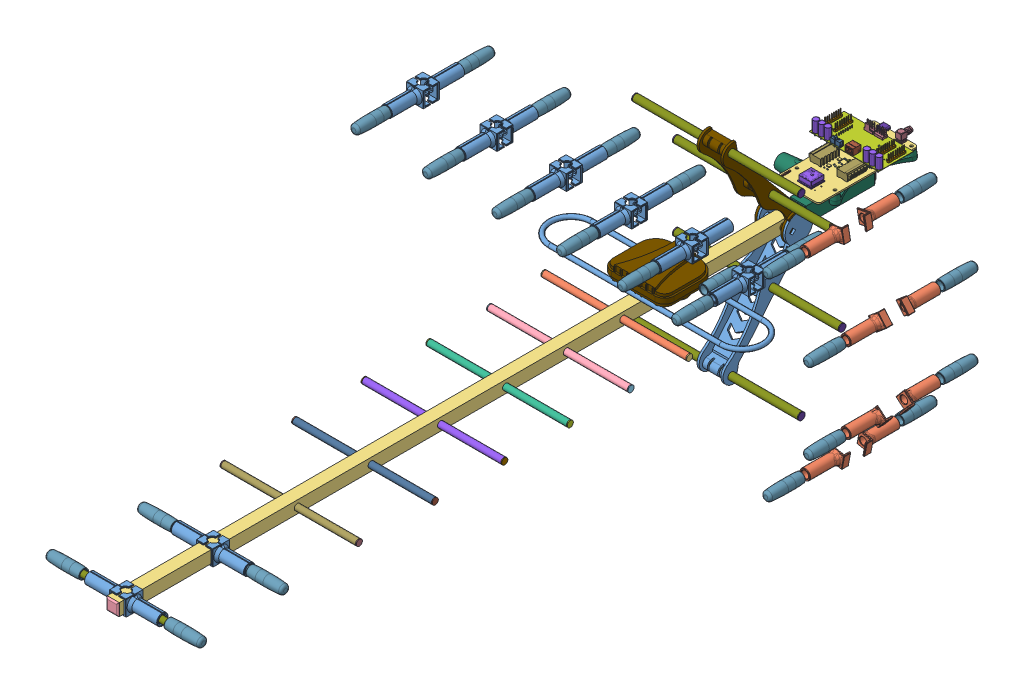
SolidWorks assembly 1. 868MHz Yagi Assembly, configuration Default. Lengths in mm.
Overall size (806.01 707.25 920.96).
274 component instances, 76 part files, 216 mates.
Components (placement in the parent):
- antenna sheath-1: antenna sheath [Default] at (505.0614 466.1407 652.9384) x (0 1 0) z (0 0 1) size (18 10 41)
- antenna sheath-2: antenna sheath [Default] at (505.0614 466.1407 652.9384) x (0 -1 0) z (0 0 1) size (18 10 41)
- antenna sheath-3: antenna sheath [Default] at (440.0614 466.1407 652.9384) x (0 1 0) z (0 0 1) size (18 10 41)
- antenna sheath-4: antenna sheath [Default] at (440.0614 466.1407 652.9384) x (0 -1 0) z (0 0 1) size (18 10 41)
- antenna sheath-5: antenna sheath [Default] at (370.0614 466.1407 652.9384) x (0 -1 0) z (0 0 1) size (18 10 41)
- antenna sheath-6: antenna sheath [Default] at (370.0614 466.1407 652.9384) x (0 1 0) z (0 0 1) size (18 10 41)
- antenna sheath-7: antenna sheath [Default] at (295.0614 466.1407 652.9384) x (0 1 0) z (0 0 1) size (18 10 41)
- antenna sheath-8: antenna sheath [Default] at (295.0614 466.1407 652.9384) x (0 -1 0) z (0 0 1) size (18 10 41)
- antenna sheath-9: antenna sheath [Default] at (215.0614 466.1407 652.9384) x (0 1 0) z (0 0 1) size (18 10 41)
- antenna sheath-10: antenna sheath [Default] at (215.0614 466.1407 652.9384) x (0 -1 0) z (0 0 1) size (18 10 41)
- antenna sheath-11: antenna sheath [Default] at (130.0614 466.1407 652.9384) x (0 1 0) z (0 0 1) size (18 10 41)
- antenna sheath-12: antenna sheath [Default] at (130.0614 466.1407 652.9384) x (0 -1 0) z (0 0 1) size (18 10 41)
- antenna sheath-13: antenna sheath [Default] at (7 0 757.5) x (0 1 0) z (1 0 0) size (18 10 41)
- antenna sheath-14: antenna sheath [Default] at (7 0 757.5) x (0 -1 0) z (1 0 0) size (18 10 41)
- antenna sheath-15: antenna sheath [Default] at (7 0 857.5) x (0 -1 0) z (1 0 0) size (18 10 41)
- antenna sheath-16: antenna sheath [Default] at (7 0 857.5) x (0 1 0) z (1 0 0) size (18 10 41)
- antenna sheath-17: antenna sheath [Default] at (505.0614 466.1407 638.9384) x (0 -1 0) z (0 0 -1) size (18 10 41)
- antenna sheath-18: antenna sheath [Default] at (505.0614 466.1407 638.9384) x (0 1 0) z (0 0 -1) size (18 10 41)
- antenna sheath-19: antenna sheath [Default] at (440.0614 466.1407 638.9384) x (0 -1 0) z (0 0 -1) size (18 10 41)
- antenna sheath-20: antenna sheath [Default] at (440.0614 466.1407 638.9384) x (0 1 0) z (0 0 -1) size (18 10 41)
- antenna sheath-21: antenna sheath [Default] at (370.0614 466.1407 638.9384) x (0 -1 0) z (0 0 -1) size (18 10 41)
- antenna sheath-22: antenna sheath [Default] at (370.0614 466.1407 638.9384) x (0 1 0) z (0 0 -1) size (18 10 41)
- antenna sheath-23: antenna sheath [Default] at (295.0614 466.1407 638.9384) x (0 1 0) z (0 0 -1) size (18 10 41)
- antenna sheath-24: antenna sheath [Default] at (295.0614 466.1407 638.9384) x (0 -1 0) z (0 0 -1) size (18 10 41)
- antenna sheath-25: antenna sheath [Default] at (215.0614 466.1407 638.9384) x (0 -1 0) z (0 0 -1) size (18 10 41)
- antenna sheath-26: antenna sheath [Default] at (215.0614 466.1407 638.9384) x (0 1 0) z (0 0 -1) size (18 10 41)
- antenna sheath-27: antenna sheath [Default] at (130.0614 466.1407 638.9384) x (0 1 0) z (0 0 -1) size (18 10 41)
- antenna sheath-28: antenna sheath [Default] at (130.0614 466.1407 638.9384) x (0 -1 0) z (0 0 -1) size (18 10 41)
- antenna sheath-29: antenna sheath [Default] at (-7 0 757.5) x (0 -1 0) z (-1 0 0) size (18 10 41)
- antenna sheath-30: antenna sheath [Default] at (-7 0 757.5) x (0 1 0) z (-1 0 0) size (18 10 41)
- antenna sheath-31: antenna sheath [Default] at (-7 0 857.5) x (0 1 0) z (-1 0 0) size (18 10 41)
- antenna sheath-32: antenna sheath [Default] at (-7 0 857.5) x (0 -1 0) z (-1 0 0) size (18 10 41)
- ground plane sheath-1: ground plane sheath [Default] at (622.1186 354.933 628.9384) x (0.186459 0.982463 0) z (0 0 -1) size (15.31 15.12 43)
- ground plane sheath-2: ground plane sheath [Default] at (622.1186 354.933 662.9384) x (-0.186459 -0.982463 0) z (0 0 1) size (15.31 15.12 43)
- ground plane sheath-3: ground plane sheath [Default] at (669.0995 419.8148 662.9384) x (-0.642788 -0.766044 0) z (0 0 1) size (15.31 15.12 43)
- ground plane sheath-4: ground plane sheath [Default] at (669.0995 419.8148 628.9384) x (0.642788 0.766044 0) z (0 0 -1) size (15.31 15.12 43)
- ground plane sheath-5: ground plane sheath [Default] at (669.0995 512.4667 662.9384) x (0.642788 -0.766044 0) z (0 0 1) size (15.31 15.12 43)
- ground plane sheath-6: ground plane sheath [Default] at (669.0995 512.4667 628.9384) x (-0.642788 0.766044 0) z (0 0 -1) size (15.31 15.12 43)
- ground plane sheath-7: ground plane sheath [Default] at (622.1186 577.3485 662.9384) x (0.186459 -0.982463 0) z (0 0 1) size (15.31 15.12 43)
- ground plane sheath-8: ground plane sheath [Default] at (622.1186 577.3485 628.9384) x (-0.186459 0.982463 0) z (0 0 -1) size (15.31 15.12 43)
- Main_Board_1_1-1: Main_Board_1_1 [Default] at (36 19.75 -38.9645) x (-1 0 0) z (0 1 0) size (70 133 15.95)
  - Main_Board_1_1_BOARD-1: Main_Board_1_1_BOARD [Default] at origin size (52 115 1.63)
  - BMP581_CMP-048-000000-2-1: BMP581_CMP-048-000000-2 [Default] at (43 50.5 0.0203) x (-0.707107 -0.707107 0) z (0 0 -1) size (2 2 0.8)
  - BMP581_CMP-048-000000-2-2: BMP581_CMP-048-000000-2 [Default] at (45.5 45.5 1.6065) x (0.707107 -0.707107 0) z (0 0 1) size (2 2 0.8)
  - RESC1609X50X30ML8T20_CMP-009-00185-4-1: RESC1609X50X30ML8T20_CMP-009-00185-4 [Default] at (40.25 53.25 0.0203) x (0 1 0) z (0 0 -1) size (1.65 0.95 0.5)
  - RESC1609X50X30ML8T20_CMP-009-00185-4-2: RESC1609X50X30ML8T20_CMP-009-00185-4 [Default] at (47.5 49 0.0203) x (0 1 0) z (0 0 -1) size (1.65 0.95 0.5)
  - RESC1609X50X30ML8T20_CMP-009-00185-4-3: RESC1609X50X30ML8T20_CMP-009-00185-4 [Default] at (41.5 53.25 0.0203) x (0 1 0) z (0 0 -1) size (1.65 0.95 0.5)
  - RESC1609X50X30ML8T20_CMP-009-00185-4-4: RESC1609X50X30ML8T20_CMP-009-00185-4 [Default] at (46.0298 49.0299 0.0203) x (0 1 0) z (0 0 -1) size (1.65 0.95 0.5)
  - RESC1609X50X30ML8T20_CMP-009-00185-4-5: RESC1609X50X30ML8T20_CMP-009-00185-4 [Default] at (45.25 53.25 0.0203) x (0 1 0) z (0 0 -1) size (1.65 0.95 0.5)
  - RESC1609X50X30ML8T20_CMP-009-00185-4-6: RESC1609X50X30ML8T20_CMP-009-00185-4 [Default] at (41.75 47.25 0.0203) x (-1 0 0) z (0 0 -1) size (1.65 0.95 0.5)
  - RESC1609X50X30ML8T20_CMP-009-00185-4-7: RESC1609X50X30ML8T20_CMP-009-00185-4 [Default] at (22.375 64 1.6065) x (-1 0 0) z (0 0 1) size (1.65 0.95 0.5)
  - RESC1609X50X30ML8T20_CMP-009-00185-4-8: RESC1609X50X30ML8T20_CMP-009-00185-4 [Default] at (23.5 62.75 1.6065) x (-1 0 0) z (0 0 1) size (1.65 0.95 0.5)
  - RESC1609X50X30ML8T20_CMP-009-00185-4-9: RESC1609X50X30ML8T20_CMP-009-00185-4 [Default] at (38.337 62.824 0.0203) x (1 0 0) z (0 0 -1) size (1.65 0.95 0.5)
  - RESC1609X50X30ML8T20_CMP-009-00185-4-10: RESC1609X50X30ML8T20_CMP-009-00185-4 [Default] at (36.322 28.829 0.0203) x (0 1 0) z (0 0 -1) size (1.65 0.95 0.5)
  - RESC1609X50X30ML8T20_CMP-009-00185-4-11: RESC1609X50X30ML8T20_CMP-009-00185-4 [Default] at (39.263 48.645 1.6065) x (0 1 0) z (0 0 1) size (1.65 0.95 0.5)
  - RESC1609X50X30ML8T20_CMP-009-00185-4-12: RESC1609X50X30ML8T20_CMP-009-00185-4 [Default] at (44.5 38.75 0.0203) x (1 0 0) z (0 0 -1) size (1.65 0.95 0.5)
  - RESC1609X50X30ML8T20_CMP-009-00185-4-13: RESC1609X50X30ML8T20_CMP-009-00185-4 [Default] at (40.914 48.645 1.6065) x (0 1 0) z (0 0 1) size (1.65 0.95 0.5)
  - RESC1609X50X30ML8T20_CMP-009-00185-4-14: RESC1609X50X30ML8T20_CMP-009-00185-4 [Default] at (30 78.25 0.0203) x (0 1 0) z (0 0 -1) size (1.65 0.95 0.5)
  - RESC1609X50X30ML8T20_CMP-009-00185-4-15: RESC1609X50X30ML8T20_CMP-009-00185-4 [Default] at (32.25 81 0.0203) x (-1 0 0) z (0 0 -1) size (1.65 0.95 0.5)
  - RESC1609X50X30ML8T20_CMP-009-00185-4-16: RESC1609X50X30ML8T20_CMP-009-00185-4 [Default] at (35 78.25 0.0203) x (0 -1 0) z (0 0 -1) size (1.65 0.95 0.5)
  - RESC1609X50X30ML8T20_CMP-009-00185-4-17: RESC1609X50X30ML8T20_CMP-009-00185-4 [Default] at (41 73.5 0.0203) x (0 1 0) z (0 0 -1) size (1.65 0.95 0.5)
  - RESC1609X50X30ML8T20_CMP-009-00185-4-18: RESC1609X50X30ML8T20_CMP-009-00185-4 [Default] at (34.5 73 0.0203) x (0 -1 0) z (0 0 -1) size (1.65 0.95 0.5)
  - RESC1609X50X30ML8T20_CMP-009-00185-4-19: RESC1609X50X30ML8T20_CMP-009-00185-4 [Default] at (36.25 73 0.0203) x (0 1 0) z (0 0 -1) size (1.65 0.95 0.5)
  - RESC1609X50X30ML8T20_CMP-009-00185-4-20: RESC1609X50X30ML8T20_CMP-009-00185-4 [Default] at (30.6372 78.25 1.6065) x (0 -1 0) z (0 0 1) size (1.65 0.95 0.5)
  - RESC1609X50X30ML8T20_CMP-009-00185-4-21: RESC1609X50X30ML8T20_CMP-009-00185-4 [Default] at (30.75 65.5 1.6065) x (0 -1 0) z (0 0 1) size (1.65 0.95 0.5)
  - RESC1609X50X30ML8T20_CMP-009-00185-4-22: RESC1609X50X30ML8T20_CMP-009-00185-4 [Default] at (39.75 77.1815 1.6065) x (0 1 0) z (0 0 1) size (1.65 0.95 0.5)
  - RESC1609X50X30ML8T20_CMP-009-00185-4-23: RESC1609X50X30ML8T20_CMP-009-00185-4 [Default] at (39.75 65.5 1.6065) x (0 1 0) z (0 0 1) size (1.65 0.95 0.5)
  - RESC1609X50X30ML8T20_CMP-009-00185-4-24: RESC1609X50X30ML8T20_CMP-009-00185-4 [Default] at (37.1957 78.25 1.6065) x (0 -1 0) z (0 0 1) size (1.65 0.95 0.5)
  - RESC1609X50X30ML8T20_CMP-009-00185-4-25: RESC1609X50X30ML8T20_CMP-009-00185-4 [Default] at (37.75 65.5 1.6065) x (0 -1 0) z (0 0 1) size (1.65 0.95 0.5)
  - RESC1609X50X30ML8T20_CMP-009-00185-4-26: RESC1609X50X30ML8T20_CMP-009-00185-4 [Default] at (38.9707 85.75 1.6065) x (-1 0 0) z (0 0 1) size (1.65 0.95 0.5)
  - RESC1609X50X30ML8T20_CMP-009-00185-4-27: RESC1609X50X30ML8T20_CMP-009-00185-4 [Default] at (38.75 72.5 1.6065) x (0 1 0) z (0 0 1) size (1.65 0.95 0.5)
  - RESC1609X50X30ML8T20_CMP-009-00185-4-28: RESC1609X50X30ML8T20_CMP-009-00185-4 [Default] at (55.245 23.495 1.6065) size (1.65 0.95 0.5)
  - RESC1609X50X30ML8T20_CMP-009-00185-4-29: RESC1609X50X30ML8T20_CMP-009-00185-4 [Default] at (55.245 25.1777 1.6065) size (1.65 0.95 0.5)
  - RESC1609X50X30ML8T20_CMP-009-00185-4-30: RESC1609X50X30ML8T20_CMP-009-00185-4 [Default] at (55.245 26.8605 1.6065) size (1.65 0.95 0.5)
  - RESC1609X50X30ML8T20_CMP-009-00185-4-31: RESC1609X50X30ML8T20_CMP-009-00185-4 [Default] at (55.245 28.5433 1.6065) size (1.65 0.95 0.5)
  - RESC1609X50X30ML8T20_CMP-009-00185-4-32: RESC1609X50X30ML8T20_CMP-009-00185-4 [Default] at (55.245 30.226 1.6065) size (1.65 0.95 0.5)
  - RESC1609X50X30ML8T20_CMP-009-00185-4-33: RESC1609X50X30ML8T20_CMP-009-00185-4 [Default] at (52.07 18.923 1.6065) size (1.65 0.95 0.5)
  - RESC1609X50X30ML8T20_CMP-009-00185-4-34: RESC1609X50X30ML8T20_CMP-009-00185-4 [Default] at (41.91 18.923 1.6065) x (-1 0 0) z (0 0 1) size (1.65 0.95 0.5)
  - RESC1609X50X30ML8T20_CMP-009-00185-4-35: RESC1609X50X30ML8T20_CMP-009-00185-4 [Default] at (52.125 55.125 1.6065) x (-1 0 0) z (0 0 1) size (1.65 0.95 0.5)
  - RESC1609X50X30ML8T20_CMP-009-00185-4-36: RESC1609X50X30ML8T20_CMP-009-00185-4 [Default] at (36.5 54.5 0.0203) x (0 1 0) z (0 0 -1) size (1.65 0.95 0.5)
  - RESC1609X50X30ML8T20_CMP-009-00185-4-37: RESC1609X50X30ML8T20_CMP-009-00185-4 [Default] at (38 54.5 0.0203) x (0 1 0) z (0 0 -1) size (1.65 0.95 0.5)
  - RESC1609X50X30ML8T20_CMP-009-00185-4-38: RESC1609X50X30ML8T20_CMP-009-00185-4 [Default] at (52.125 57.375 1.6065) x (-1 0 0) z (0 0 1) size (1.65 0.95 0.5)
  - RESC1609X50X30ML8T20_CMP-009-00185-4-39: RESC1609X50X30ML8T20_CMP-009-00185-4 [Default] at (41.75 45.75 0.0203) x (1 0 0) z (0 0 -1) size (1.65 0.95 0.5)
  - RESC1609X50X30ML8T20_CMP-009-00185-4-40: RESC1609X50X30ML8T20_CMP-009-00185-4 [Default] at (41.75 44.25 0.0203) x (1 0 0) z (0 0 -1) size (1.65 0.95 0.5)
  - FP-0603-L_1_6_0_15-W_0_81-IPC_C_CMP-001-00088-6-1: FP-0603-L_1_6_0_15-W_0_81-IPC_C_CMP-001-00088-6 [Default] at (42.75 53.25 0.0203) x (0 -1 0) z (0 0 -1) size (1.65 0.86 0.94)
  - FP-0603-L_1_6_0_15-W_0_81-IPC_C_CMP-001-00088-6-2: FP-0603-L_1_6_0_15-W_0_81-IPC_C_CMP-001-00088-6 [Default] at (46 48 1.6065) x (0 -1 0) z (0 0 1) size (1.65 0.86 0.94)
  - FP-0603-L_1_6_0_15-W_0_81-IPC_C_CMP-001-00088-6-3: FP-0603-L_1_6_0_15-W_0_81-IPC_C_CMP-001-00088-6 [Default] at (44 53.25 0.0203) x (0 -1 0) z (0 0 -1) size (1.65 0.86 0.94)
  - FP-0603-L_1_6_0_15-W_0_81-IPC_C_CMP-001-00088-6-4: FP-0603-L_1_6_0_15-W_0_81-IPC_C_CMP-001-00088-6 [Default] at (44.75 48 1.6065) x (0 -1 0) z (0 0 1) size (1.65 0.86 0.94)
  - FP-0603-L_1_6_0_15-W_0_81-IPC_C_CMP-001-00088-6-5: FP-0603-L_1_6_0_15-W_0_81-IPC_C_CMP-001-00088-6 [Default] at (29.21 30.861 1.6065) x (0.707107 0.707107 0) z (0 0 1) size (1.65 0.86 0.94)
  - FP-0603-L_1_6_0_15-W_0_81-IPC_C_CMP-001-00088-6-6: FP-0603-L_1_6_0_15-W_0_81-IPC_C_CMP-001-00088-6 [Default] at (32.25 75.75 0.0203) x (1 0 0) z (0 0 -1) size (1.65 0.86 0.94)
  - FP-0603-L_1_6_0_15-W_0_81-IPC_C_CMP-001-00088-6-7: FP-0603-L_1_6_0_15-W_0_81-IPC_C_CMP-001-00088-6 [Default] at (44 78.5 0.0203) x (0 1 0) z (0 0 -1) size (1.65 0.86 0.94)
  - FP-0603-L_1_6_0_15-W_0_81-IPC_C_CMP-001-00088-6-8: FP-0603-L_1_6_0_15-W_0_81-IPC_C_CMP-001-00088-6 [Default] at (42.5 73.5 0.0203) x (0 -1 0) z (0 0 -1) size (1.65 0.86 0.94)
  - FP-0603-L_1_6_0_15-W_0_81-IPC_C_CMP-001-00088-6-9: FP-0603-L_1_6_0_15-W_0_81-IPC_C_CMP-001-00088-6 [Default] at (44 73.5 0.0203) x (0 -1 0) z (0 0 -1) size (1.65 0.86 0.94)
  - FP-0603-L_1_6_0_15-W_0_81-IPC_C_CMP-001-00088-6-10: FP-0603-L_1_6_0_15-W_0_81-IPC_C_CMP-001-00088-6 [Default] at (42.5 78.5 0.0203) x (0 1 0) z (0 0 -1) size (1.65 0.86 0.94)
  - FP-0603-L_1_6_0_15-W_0_81-IPC_C_CMP-001-00088-6-11: FP-0603-L_1_6_0_15-W_0_81-IPC_C_CMP-001-00088-6 [Default] at (38.375 39.625 0.0203) x (0 -1 0) z (0 0 -1) size (1.65 0.86 0.94)
  - FP-0603-L_1_6_0_15-W_0_81-IPC_C_CMP-001-00088-6-12: FP-0603-L_1_6_0_15-W_0_81-IPC_C_CMP-001-00088-6 [Default] at (40.25 45 1.6065) x (0 -1 0) z (0 0 1) size (1.65 0.86 0.94)
  - FP-0603-L_1_6_0_15-W_0_81-IPC_C_CMP-001-00088-6-13: FP-0603-L_1_6_0_15-W_0_81-IPC_C_CMP-001-00088-6 [Default] at (51.816 32.385 1.6065) x (-1 0 0) z (0 0 1) size (1.65 0.86 0.94)
  - FP-0603-L_1_6_0_15-W_0_81-IPC_C_CMP-001-00088-6-14: FP-0603-L_1_6_0_15-W_0_81-IPC_C_CMP-001-00088-6 [Default] at (37.125 39.625 0.0203) x (0 -1 0) z (0 0 -1) size (1.65 0.86 0.94)
  - FP-0603-L_1_6_0_15-W_0_81-IPC_C_CMP-001-00088-6-15: FP-0603-L_1_6_0_15-W_0_81-IPC_C_CMP-001-00088-6 [Default] at (28.321 31.75 1.6065) x (0.707107 0.707107 0) z (0 0 1) size (1.65 0.86 0.94)
  - FP-0603-L_1_6_0_15-W_0_81-IPC_C_CMP-001-00088-6-16: FP-0603-L_1_6_0_15-W_0_81-IPC_C_CMP-001-00088-6 [Default] at (40.64 22.733 1.6065) x (0 1 0) z (0 0 1) size (1.65 0.86 0.94)
  - FP-0603-L_1_6_0_15-W_0_81-IPC_C_CMP-001-00088-6-17: FP-0603-L_1_6_0_15-W_0_81-IPC_C_CMP-001-00088-6 [Default] at (39.243 22.733 1.6065) x (0 1 0) z (0 0 1) size (1.65 0.86 0.94)
  - FP-0603-L_1_6_0_15-W_0_81-IPC_C_CMP-001-00088-6-18: FP-0603-L_1_6_0_15-W_0_81-IPC_C_CMP-001-00088-6 [Default] at (20.955 34.798 1.6065) size (1.65 0.86 0.94)
  - FP-0603-L_1_6_0_15-W_0_81-IPC_C_CMP-001-00088-6-19: FP-0603-L_1_6_0_15-W_0_81-IPC_C_CMP-001-00088-6 [Default] at (37.338 22.733 1.6065) x (0 -1 0) z (0 0 1) size (1.65 0.86 0.94)
  - FP-0603-L_1_6_0_15-W_0_81-IPC_C_CMP-001-00088-6-20: FP-0603-L_1_6_0_15-W_0_81-IPC_C_CMP-001-00088-6 [Default] at (51.181 30.861 1.6065) size (1.65 0.86 0.94)
  - FP-0603-L_1_6_0_15-W_0_81-IPC_C_CMP-001-00088-6-21: FP-0603-L_1_6_0_15-W_0_81-IPC_C_CMP-001-00088-6 [Default] at (31.496 39.624 0.0203) x (0 -1 0) z (0 0 -1) size (1.65 0.86 0.94)
  - FP-0603-L_1_6_0_15-W_0_81-IPC_C_CMP-001-00088-6-22: FP-0603-L_1_6_0_15-W_0_81-IPC_C_CMP-001-00088-6 [Default] at (30.353 39.624 0.0203) x (0 -1 0) z (0 0 -1) size (1.65 0.86 0.94)
  - FP-0603-L_1_6_0_15-W_0_81-IPC_C_CMP-001-00088-6-23: FP-0603-L_1_6_0_15-W_0_81-IPC_C_CMP-001-00088-6 [Default] at (51.689 24.4251 1.6065) x (0 -1 0) z (0 0 1) size (1.65 0.86 0.94)
  - FP-0603-L_1_6_0_15-W_0_81-IPC_C_CMP-001-00088-6-24: FP-0603-L_1_6_0_15-W_0_81-IPC_C_CMP-001-00088-6 [Default] at (34.5 92.75 0.0203) x (0 -1 0) z (0 0 -1) size (1.65 0.86 0.94)
  - FP-0603-L_1_6_0_15-W_0_81-IPC_C_CMP-001-00088-6-25: FP-0603-L_1_6_0_15-W_0_81-IPC_C_CMP-001-00088-6 [Default] at (39.988 60.411 0.0203) x (0 1 0) z (0 0 -1) size (1.65 0.86 0.94)
  - FP-0603-L_1_6_0_15-W_0_81-IPC_C_CMP-001-00088-6-26: FP-0603-L_1_6_0_15-W_0_81-IPC_C_CMP-001-00088-6 [Default] at (33.511 61.3 0.0203) x (0 1 0) z (0 0 -1) size (1.65 0.86 0.94)
  - FP-0603-L_1_6_0_15-W_0_81-IPC_C_CMP-001-00088-6-27: FP-0603-L_1_6_0_15-W_0_81-IPC_C_CMP-001-00088-6 [Default] at (35.67 62.57 0.0203) x (-1 0 0) z (0 0 -1) size (1.65 0.86 0.94)
  - FP-0603-L_1_6_0_15-W_0_81-IPC_C_CMP-001-00088-6-28: FP-0603-L_1_6_0_15-W_0_81-IPC_C_CMP-001-00088-6 [Default] at (33.782 37.592 0.0203) x (1 0 0) z (0 0 -1) size (1.65 0.86 0.94)
  - FP-0603-L_1_6_0_15-W_0_81-IPC_C_CMP-001-00088-2-1: FP-0603-L_1_6_0_15-W_0_81-IPC_C_CMP-001-00088-2 [Default] at (37 117.5 0.0203) x (1 0 0) z (0 0 -1) size (1.6 0.81 0.9)
  - FP-0603-L_1_6_0_15-W_0_81-IPC_C_CMP-001-00088-2-2: FP-0603-L_1_6_0_15-W_0_81-IPC_C_CMP-001-00088-2 [Default] at (37 96.75 0.0203) x (-1 0 0) z (0 0 -1) size (1.6 0.81 0.9)
  - FP-0603-L_1_6_0_15-W_0_81-IPC_C_CMP-001-00088-2-3: FP-0603-L_1_6_0_15-W_0_81-IPC_C_CMP-001-00088-2 [Default] at (37 101.75 0.0203) x (-1 0 0) z (0 0 -1) size (1.6 0.81 0.9)
  - FP-0603-L_1_6_0_15-W_0_81-IPC_C_CMP-001-00088-2-4: FP-0603-L_1_6_0_15-W_0_81-IPC_C_CMP-001-00088-2 [Default] at (42 96.75 0.0203) x (1 0 0) z (0 0 -1) size (1.6 0.81 0.9)
  - FP-0603-L_1_6_0_15-W_0_81-IPC_C_CMP-001-00088-2-5: FP-0603-L_1_6_0_15-W_0_81-IPC_C_CMP-001-00088-2 [Default] at (42 101.75 0.0203) x (1 0 0) z (0 0 -1) size (1.6 0.81 0.9)
  - QUEC-L80-M39-12_V_CMP-021-00008-3-1: QUEC-L80-M39-12_V_CMP-021-00008-3 [Default] at (36.48 107 1.6065) x (0 1 0) z (0 0 1) size (16 16 6.95)
  - RESC1608X55X25ML10T15_CMP-009-00177-3-1: RESC1608X55X25ML10T15_CMP-009-00177-3 [Default] at (37.3293 68.1458 0.0203) x (1 0 0) z (0 0 -1) size (1.7 0.9 0.55)
  - RESC1608X55X25ML10T15_CMP-009-00177-3-2: RESC1608X55X25ML10T15_CMP-009-00177-3 [Default] at (27.051 22.733 1.6065) x (0 -1 0) z (0 0 1) size (1.7 0.9 0.55)
  - RESC1608X55X25ML10T15_CMP-009-00177-3-3: RESC1608X55X25ML10T15_CMP-009-00177-3 [Default] at (34.5 88.6457 0.0203) x (0 1 0) z (0 0 -1) size (1.7 0.9 0.55)
  - RESC1608X55X25ML10T15_CMP-009-00177-3-4: RESC1608X55X25ML10T15_CMP-009-00177-3 [Default] at (20.955 36.322 1.6065) x (-1 0 0) z (0 0 1) size (1.7 0.9 0.55)
  - AO-SOT-23-3L_V_CMP-013-00037-1-1: AO-SOT-23-3L_V_CMP-013-00037-1 [Default] at (33.25 69.3457 0.0203) x (0 1 0) z (0 0 -1) size (3 3.1 1.25)
  - LED_WS2812-2020_CMP-002-000000-1-1: LED_WS2812-2020_CMP-002-000000-1 [Default] at (58.778 112.3103 1.6065) x (-1 0 0) z (0 0 1) size (2.2 2 0.84)
  - LED_WS2812-2020_CMP-002-000000-1-2: LED_WS2812-2020_CMP-002-000000-1 [Default] at (58.778 109.728 1.6065) x (-1 0 0) z (0 0 1) size (2.2 2 0.84)
  - LED_WS2812-2020_CMP-002-000000-1-3: LED_WS2812-2020_CMP-002-000000-1 [Default] at (58.778 117.475 1.6065) x (-1 0 0) z (0 0 1) size (2.2 2 0.84)
  - LED_WS2812-2020_CMP-002-000000-1-4: LED_WS2812-2020_CMP-002-000000-1 [Default] at (58.778 114.8927 1.6065) x (-1 0 0) z (0 0 1) size (2.2 2 0.84)
  - FP-S8411-45R-MFG_CMP-002-00079-1-1: FP-S8411-45R-MFG_CMP-002-00079-1 [Default] at (25.527 110.165 0.0203) x (-1 0 0) z (0 0 -1) size (14.75 19.2 5.45)
  - MCC-SOD-123FL_V_CMP-004-00034-1-1: MCC-SOD-123FL_V_CMP-004-00034-1 [Default] at (29.4186 89.9257 0.0203) x (0 1 0) z (0 0 -1) size (3.7 1.9 1.2)
  - MCC-SOD-123FL_V_CMP-004-00034-1-2: MCC-SOD-123FL_V_CMP-004-00034-1 [Default] at (31.8228 90.158 0.0203) x (0 1 0) z (0 0 -1) size (3.7 1.9 1.2)
  - FP-FTSH-107-01-F-DV-K-MFG_CMP-002-00087-1-1: FP-FTSH-107-01-F-DV-K-MFG_CMP-002-00087-1 [Default] at (44.25 55.75 1.6065) x (-1 0 0) z (0 0 1) size (8.97 5.87 6.44)
  - FP-SOT23-IPC_C_CMP-013-00038-1-1: FP-SOT23-IPC_C_CMP-013-00038-1 [Default] at (26.924 48.006 0.0203) x (-1 0 0) z (0 0 -1) size (2.82 2.9 1.25)
  - SOT95P245X110-5N_CMP-011-00013-1-1: SOT95P245X110-5N_CMP-011-00013-1 [Default] at (33.9165 78.2 1.6065) size (1.4 3 1.05)
  - SOT95P245X110-5N_CMP-011-00013-1-2: SOT95P245X110-5N_CMP-011-00013-1 [Default] at (34.75 65.5 1.6065) size (1.4 3 1.05)
  - THRMC1608X95N_CMP-038-000000-2-1: THRMC1608X95N_CMP-038-000000-2 [Default] at (29.8107 70.6457 0.0203) x (1 0 0) z (0 0 -1) size (1.6 0.8 0.45)
  - FP-CRCW0603-e3-IPC_C_0603WAF220JT5E-2-1: FP-CRCW0603-e3-IPC_C_0603WAF220JT5E-2 [Default] at (58.75 121.5 1.6065) x (-1 0 0) z (0 0 1) size (1.55 0.85 0.5)
  - SOT95P230X110-3N_CMP-013-000004-1-1: SOT95P230X110-3N_CMP-013-000004-1 [Default] at (37.5 77.75 0.0203) x (0 -1 0) z (0 0 -1) size (2.4 2.9 0.95)
  - SSM6J507NULF_CMP-013-000003-10-1: SSM6J507NULF_CMP-013-000003-10 [Default] at (38.75 73.675 0.0203) x (0 -1 0) z (0 0 -1) size (2 2.22 0.9)
  - AON7544_CMP-089-000000-2-1: AON7544_CMP-089-000000-2 [Default] at (41.225 81.7657 1.6065) x (0 -1 0) z (0 0 1) size (3.13 3.23 1)
  - AON7544_CMP-089-000000-2-2: AON7544_CMP-089-000000-2 [Default] at (41.39 69.25 1.6065) x (0 -1 0) z (0 0 1) size (3.13 3.23 1)
  - FP-BLM18-0_15-0_1-t0_6-IPC_B_CMP-006-00021-1-1: FP-BLM18-0_15-0_1-t0_6-IPC_B_CMP-006-00021-1 [Default] at (51.689 27.4731 1.6065) x (0 1 0) z (0 0 1) size (1.6 0.8 0.7)
  - FP-BLM18-0_15-0_1-t0_6-IPC_B_CMP-006-00021-1-2: FP-BLM18-0_15-0_1-t0_6-IPC_B_CMP-006-00021-1 [Default] at (29.591 37.719 0.0203) x (-1 0 0) z (0 0 -1) size (1.6 0.8 0.7)
  - FP-LTST-C190GKT-MFG_CMP-00026-00001-1-1: FP-LTST-C190GKT-MFG_CMP-00026-00001-1 [Default] at (58.75 119.75 1.6065) size (1.6 0.8 0.9)
  - FP-LTST-C190GKT-MFG_CMP-00026-00001-1-2: FP-LTST-C190GKT-MFG_CMP-00026-00001-1 [Default] at (42.25 86 1.6065) x (-1 0 0) z (0 0 1) size (1.6 0.8 0.9)
  - FP-LTST-C190GKT-MFG_CMP-00026-00001-1-3: FP-LTST-C190GKT-MFG_CMP-00026-00001-1 [Default] at (35.75 72.5 1.6065) x (0 -1 0) z (0 0 1) size (1.6 0.8 0.9)
  - MCC-SOD123_V_CMP-004-00005-3-1: MCC-SOD123_V_CMP-004-00005-3 [Default] at (41.5 76 0.0203) x (1 0 0) z (0 0 -1) size (2.7 1.6 1.35)
  - FP-CL10-IPC_B_CMP-001-00087-1-1: FP-CL10-IPC_B_CMP-001-00087-1 [Default] at (28.702 39.243 1.6065) x (-0.707107 0.707107 0) z (0 0 1) size (1.6 0.8 0.9)
  - FP-CL10-IPC_B_CMP-001-00087-1-2: FP-CL10-IPC_B_CMP-001-00087-1 [Default] at (29.21 43.561 1.6065) x (-0.707107 -0.707107 0) z (0 0 1) size (1.6 0.8 0.9)
  - FP-CL10-IPC_B_CMP-001-00086-2-1: FP-CL10-IPC_B_CMP-001-00086-2 [Default] at (32.258 46.228 1.6065) x (-0.707107 0.707107 0) z (0 0 1) size (1.6 0.8 0.9)
  - FP-CL10-IPC_B_CMP-001-00086-2-2: FP-CL10-IPC_B_CMP-001-00086-2 [Default] at (34.036 47.752 1.6065) x (-0.707107 0.707107 0) z (0 0 1) size (1.6 0.8 0.9)
  - CAPPM3528X210N_CMP-054-000000-2-1: CAPPM3528X210N_CMP-054-000000-2 [Default] at (43.5 65.6458 0.0203) x (0 1 0) z (0 0 -1) size (3.5 2.85 2.1)
  - SLIN-PPPC081LFBN-RC_V_CMP-002-00028-2-1: SLIN-PPPC081LFBN-RC_V_CMP-002-00028-2 [Default] at (16.95 50 1.6065) x (0 -1 0) z (0 0 1) size (20.82 2.54 11.7)
  - SLIN-PPPC081LFBN-RC_V_CMP-002-00028-2-2: SLIN-PPPC081LFBN-RC_V_CMP-002-00028-2 [Default] at (55.05 50 1.6065) x (0 -1 0) z (0 0 1) size (20.82 2.54 11.7)
  - KXG1203C_CMP-059-000000-1-1: KXG1203C_CMP-059-000000-1 [Default] at (26.543 53.086 1.6065) x (0 1 0) z (0 0 1) size (12 12 14)
  - SHDR12W80P700X350_2X6_2170X1400X850P_CMP-062-000000-2-1: SHDR12W80P700X350_2X6_2170X1400X850P_CMP-062-000000-2 [Default] at (53.75 67.75 1.6065) x (0 1 0) z (0 0 1) size (21.7 14.3 12)
  - SHDR12W80P700X350_2X6_2170X1400X850P_CMP-062-000000-2-2: SHDR12W80P700X350_2X6_2170X1400X850P_CMP-062-000000-2 [Default] at (18.25 85 1.6065) x (0 -1 0) z (0 0 1) size (21.7 14.3 12)
  - PCBSMAFRAHT_CMP-070-000000-2-1: PCBSMAFRAHT_CMP-070-000000-2 [Default] at (24.857 14.951 1.6065) x (-1 0 0) z (0 0 1) size (9.21 15.6 13.8)
  - FP-BNO085-MFG_CMP-010-00028-1-1: FP-BNO085-MFG_CMP-010-00028-1 [Default] at (36.5 59 0.0203) x (-1 0 0) z (0 0 -1) size (3.8 5.2 1.18)
  - SOT65P210X110-5N_CMP-064-000000-3-1: SOT65P210X110-5N_CMP-064-000000-3 [Default] at (32.25 78.5 0.0203) x (0 -1 0) z (0 0 -1) size (2.12 2 1.1)
  - LoRa-CC68-868-TCXO-Footprint-1_CMP-00025-00003-3-1: LoRa-CC68-868-TCXO-Footprint-1_CMP-00025-00003-3 [Default] at (25.146 27.94 0.0203) x (-1 0 0) z (0 0 -1) size (16 16 2.1)
  - VALCON_CSP-USC16-TR_CMP-042-000000-3-1: VALCON_CSP-USC16-TR_CMP-042-000000-3 [Default] at (47 16.891 1.6065) size (8.94 7.75 4.26)
  - FP-NX3225GA-MFG_CMP-003-00030-1-1: FP-NX3225GA-MFG_CMP-003-00030-1 [Default] at (30.734 41.402 1.6065) x (-0.707107 -0.707107 0) z (0 0 1) size (3.21 2.51 0.9)
  - FP-NX3215SA-MFG_CMP-003-00031-1-1: FP-NX3215SA-MFG_CMP-003-00031-1 [Default] at (35.052 44.958 1.6065) x (-0.707107 -0.707107 0) z (0 0 1) size (3.21 1.51 0.9)
  - SOIC127P790X216-8N_CMP-040-000000-2-1: SOIC127P790X216-8N_CMP-040-000000-2 [Default] at (39.878 35.687 0.0203) x (-1 0 0) z (0 0 -1) size (7.9 5.28 2.16)
  - D0008A_L_CMP-019-00052-1-1: D0008A_L_CMP-019-00052-1 [Default] at (39.009 90.1617 0.0203) x (1 0 0) z (0 0 -1) size (6 4.9 1.63)
  - CKCP-PTS645S_V_CMP-011-00016-1-1: CKCP-PTS645S_V_CMP-011-00016-1 [Default] at (21.131 24.257 1.6065) x (-1 0 0) z (0 0 1) size (9 6 4.3)
  - CKCP-PTS645S_V_CMP-011-00016-1-2: CKCP-PTS645S_V_CMP-011-00016-1 [Default] at (21.131 31.115 1.6065) x (-1 0 0) z (0 0 1) size (9 6 4.3)
  - MOLX-473521001_V_CMP-002-00077-1-1: MOLX-473521001_V_CMP-002-00077-1 [Default] at (48.7 25 0.0203) x (0 -1 0) z (0 0 -1) size (14.1 15.2 1.89)
  - QFP50P1600X1600X160-100N_CMP-028-000000-1-1: QFP50P1600X1600X160-100N_CMP-028-000000-1 [Default] at (40 34 1.6065) x (0.707107 -0.707107 0) z (0 0 1) size (16 16 1.6)
- Ground_Station_-_Copy_for_Callum_and_Yiannis-1: Ground_Station_-_Copy_for_Callum_and_Yiannis [Default] at (39.9201 32.3864 -9.4584) x (-1 0 0) z (0 1 0) size (80 40 21.5)
  - Ground_Station_-_Copy_for_Callum_and_Yiannis_BOARD-1: Ground_Station_-_Copy_for_Callum_and_Yiannis_BOARD [Default] at origin size (80 40 0.41)
  - CAPPR55-250-1120X630X1220_CMP-001-00030-7-1: CAPPR55-250-1120X630X1220_CMP-001-00030-7 [Default] at (76.2 36.068 0.4013) x (0 1 0) z (0 0 1) size (6.31 6.3 16.21)
  - CAPPR55-250-1120X630X1220_CMP-001-00030-7-2: CAPPR55-250-1120X630X1220_CMP-001-00030-7 [Default] at (62.484 36.088 0.4013) x (0 1 0) z (0 0 1) size (6.31 6.3 16.21)
  - CAPPR55-250-1120X630X1220_CMP-001-00030-7-3: CAPPR55-250-1120X630X1220_CMP-001-00030-7 [Default] at (69.342 36.068 0.4013) x (0 1 0) z (0 0 1) size (6.31 6.3 16.21)
  - CAPPR55-250-1120X630X1220_CMP-001-00030-7-4: CAPPR55-250-1120X630X1220_CMP-001-00030-7 [Default] at (17.526 36.1117 0.4013) x (0 1 0) z (0 0 1) size (6.31 6.3 16.21)
  - CAPPR55-250-1120X630X1220_CMP-001-00030-7-5: CAPPR55-250-1120X630X1220_CMP-001-00030-7 [Default] at (3.556 36.0917 0.4013) x (0 1 0) z (0 0 1) size (6.31 6.3 16.21)
  - CAPPR55-250-1120X630X1220_CMP-001-00030-7-6: CAPPR55-250-1120X630X1220_CMP-001-00030-7 [Default] at (10.668 36.1117 0.4013) x (0 1 0) z (0 0 1) size (6.31 6.3 16.21)
  - TMC2209-Footprint-1_CMP-024-00000-2-1: TMC2209-Footprint-1_CMP-024-00000-2 [Default] at (65 25 0.4013) size (14.02 19.91 11.18)
  - TMC2209-Footprint-1_CMP-024-00000-2-2: TMC2209-Footprint-1_CMP-024-00000-2 [Default] at (3.556 25 0.4013) size (14.02 19.91 11.18)
  - ESWI-EG1218_V_CMP-011-00006-2-1: ESWI-EG1218_V_CMP-011-00006-2 [Default] at (51.054 37.338 0.4013) x (-1 0 0) z (0 0 1) size (11.6 4 12.1)
  - RESC1609X50X30ML8T20_CMP-009-00185-4-1: RESC1609X50X30ML8T20_CMP-009-00185-4 [Default] at (25.146 14.54 0.4013) x (0 1 0) z (0 0 1) size (1.65 0.95 0.5)
  - PHOE-1803277_V_CMP-002-00014-2-1: PHOE-1803277_V_CMP-002-00014-2 [Default] at (34.544 31.75 0.4013) x (-1 0 0) z (0 0 1) size (9.01 9.3 10.65)
  - FP-M20-9990846-MFG_CMP-15831-000033-1-1: FP-M20-9990846-MFG_CMP-15831-000033-1 [Default] at (59.05 20.574 0.0102) x (0 -1 0) z (0 0 -1) size (20.36 2.58 12.15)
  - FP-M20-9990846-MFG_CMP-15831-000033-1-2: FP-M20-9990846-MFG_CMP-15831-000033-1 [Default] at (20.95 20 0.0102) x (0 1 0) z (0 0 -1) size (20.36 2.58 12.15)
  - FP-47053-1000-MFG_CMP-002-00086-1-1: FP-47053-1000-MFG_CMP-002-00086-1 [Default] at (33.782 3.938 0.4013) x (-1 0 0) z (0 0 1) size (10.28 5.91 13.57)
  - FP-47053-1000-MFG_CMP-002-00086-1-2: FP-47053-1000-MFG_CMP-002-00086-1 [Default] at (45.212 4.064 0.4013) size (10.28 5.91 13.57)
- 868MHz Yagi Tip Covers-1: 868MHz Yagi Tip Covers [Default] at (-89 0 857.5) x (0 -0.979243 -0.20269) z (0 -0.20269 0.979243) size (12 40 12)
- 868MHz Yagi Tip Covers-2: 868MHz Yagi Tip Covers [Default] at (89 0 857.5) x (0 -0.750054 0.661376) z (0 -0.661376 -0.750054) size (12 40 12)
- 868MHz Yagi Tip Covers-3: 868MHz Yagi Tip Covers [Default] at (83.5 0 757.5) x (0 0.662519 0.749045) z (0 -0.749045 0.662519) size (12 40 12)
- 868MHz Yagi Tip Covers-4: 868MHz Yagi Tip Covers [Default] at (130.0614 466.1407 725.4384) x (-0.904433 -0.426616 0) z (0.426616 -0.904433 0) size (12 40 12)
- 868MHz Yagi Tip Covers-5: 868MHz Yagi Tip Covers [Default] at (215.0614 466.1407 727.9384) x (-0.904857 -0.425715 0) z (0.425715 -0.904857 0) size (12 40 12)
- 868MHz Yagi Tip Covers-6: 868MHz Yagi Tip Covers [Default] at (295.0614 466.1407 727.9384) x (-0.903571 -0.428439 0) z (0.428439 -0.903571 0) size (12 40 12)
- 868MHz Yagi Tip Covers-7: 868MHz Yagi Tip Covers [Default] at (370.0614 466.1407 728.4384) x (-0.957892 0.28713 0) z (-0.28713 -0.957892 0) size (12 40 12)
- 868MHz Yagi Tip Covers-8: 868MHz Yagi Tip Covers [Default] at (440.0614 466.1407 728.4384) x (-0.975464 -0.220159 0) z (0.220159 -0.975464 0) size (12 40 12)
- 868MHz Yagi Tip Covers-9: 868MHz Yagi Tip Covers [Default] at (505.0614 466.1407 730.9384) x (-0.847367 0.531007 0) z (-0.531007 -0.847367 0) size (12 40 12)
- 868MHz Yagi Tip Covers-10: 868MHz Yagi Tip Covers [Default] at (622.1186 354.933 742.9384) x (-0.989737 -0.142899 0) z (0.142899 -0.989737 0) size (12 40 12)
- 868MHz Yagi Tip Covers-11: 868MHz Yagi Tip Covers [Default] at (669.0995 419.8148 742.9384) x (-0.995957 -0.089831 0) z (0.089831 -0.995957 0) size (12 40 12)
- 868MHz Yagi Tip Covers-12: 868MHz Yagi Tip Covers [Default] at (669.0995 512.4667 742.9384) x (-0.944802 -0.327641 0) z (0.327641 -0.944802 0) size (12 40 12)
- 868MHz Yagi Tip Covers-13: 868MHz Yagi Tip Covers [Default] at (622.1186 577.3485 742.9384) x (-0.99421 -0.107451 0) z (0.107451 -0.99421 0) size (12 40 12)
- 868MHz Yagi Tip Covers-14: 868MHz Yagi Tip Covers [Default] at (622.1186 577.3485 548.9384) x (0.930341 -0.366696 0) z (-0.366696 -0.930341 0) size (12 40 12)
- 868MHz Yagi Tip Covers-15: 868MHz Yagi Tip Covers [Default] at (669.0995 512.4667 548.9384) x (0.970614 -0.240641 0) z (-0.240641 -0.970614 0) size (12 40 12)
- 868MHz Yagi Tip Covers-16: 868MHz Yagi Tip Covers [Default] at (505.0614 466.1407 560.9384) x (0.988874 0.148758 0) z (0.148758 -0.988874 0) size (12 40 12)
- 868MHz Yagi Tip Covers-17: 868MHz Yagi Tip Covers [Default] at (475.435 450.7404 627.737) x (0.411933 0.911214 0) z (0.911214 -0.411933 0) size (12 40 12)
- 868MHz Yagi Tip Covers-18: 868MHz Yagi Tip Covers [Default] at (370.0614 466.1407 563.4384) x (0.998037 -0.062632 0) z (-0.062632 -0.998037 0) size (12 40 12)
- 868MHz Yagi Tip Covers-19: 868MHz Yagi Tip Covers [Default] at (295.0614 466.1407 563.9384) x (0.958701 0.284417 0) z (0.284417 -0.958701 0) size (12 40 12)
- 868MHz Yagi Tip Covers-20: 868MHz Yagi Tip Covers [Default] at (215.0614 466.1407 563.9384) x (0.996486 0.083765 0) z (0.083765 -0.996486 0) size (12 40 12)
- 868MHz Yagi Tip Covers-21: 868MHz Yagi Tip Covers [Default] at (130.0614 466.1407 566.4384) x (-0.125203 -0.992131 0) z (-0.992131 0.125203 0) size (12 40 12)
- 868MHz Yagi Tip Covers-22: 868MHz Yagi Tip Covers [Default] at (-83.5 0 757.5) x (0 0.981037 -0.193819) z (0 -0.193819 -0.981037) size (12 40 12)
- 868MHz Yagi Tip Covers-23: 868MHz Yagi Tip Covers [Default] at (669.0995 419.8148 548.9384) x (0.092406 0.995721 0) z (0.995721 -0.092406 0) size (12 40 12)
- 868MHz Yagi Tip Covers-24: 868MHz Yagi Tip Covers [Default] at (622.1186 354.933 548.9384) x (0.568397 0.822755 0) z (0.822755 -0.568397 0) size (12 40 12)
- Yagi Adaptor-1: Yagi Adaptor [Default] at (0 0 4.0355) x (0 -1 0) z (-1 0 0) size (29 117.3 86)
- naked_antenna_v1-1: naked_antenna_v1 [Default] at (0 0 43) x (0 0 -1) z (1 0 0) size (874 241.1 250)
  - naked_antenna_v1.step-1: naked_antenna_v1.step [Default] at origin size (874 241.1 250)
    - Reflector.step-1: Reflector.step [Default] at origin size (101.04 241.1 192)
      - struct.step-1: struct.step [Default] at origin size (101.04 136.55 192)
        - element.step-1: element.step [Default] at origin size (8 8 192)
          - extrusion_1.step-1: extrusion_1.step [Default] at origin size (8 8 190)
          - end cap_1.step-1: end cap_1.step [Default] at origin size (8 8 3)
          - end cap_1.step-2: end cap_1.step [Default] at (0 222.4155 0) x (1 0 0) z (0 0 -1) size (8 8 3)
        - element_1.step-1: element_1.step [Default] at (30 0 0) size (8 8 192)
          - extrusion_1.step-1: extrusion_1.step [Default] at (16.9809 -64.8818 0) size (8 8 190)
          - end cap_1.step-1: end cap_1.step [Default] at (16.9809 -64.8818 0) size (8 8 3)
          - end cap_1.step-2: end cap_1.step [Default] at (16.9809 157.5337 0) x (1 0 0) z (0 0 -1) size (8 8 3)
        - struct-0.step-1: struct-0.step [Default] at origin size (101.04 136.55 35)
      - struct_1.step-1: struct_1.step [Default] x (1 0 0) z (0 0 -1) size (101.04 136.55 192)
        - element_2.step-1: element_2.step [Default] at origin size (8 8 192)
          - extrusion_1.step-1: extrusion_1.step [Default] at origin size (8 8 190)
          - end cap_1.step-1: end cap_1.step [Default] at origin size (8 8 3)
          - end cap_1.step-2: end cap_1.step [Default] at (0 222.4155 0) x (1 0 0) z (0 0 -1) size (8 8 3)
        - element_3.step-1: element_3.step [Default] at (30 0 0) size (8 8 192)
          - extrusion_1.step-1: extrusion_1.step [Default] at (16.9809 -64.8818 0) size (8 8 190)
          - end cap_1.step-1: end cap_1.step [Default] at (16.9809 -64.8818 0) size (8 8 3)
          - end cap_1.step-2: end cap_1.step [Default] at (16.9809 157.5337 0) x (1 0 0) z (0 0 -1) size (8 8 3)
        - struct_1-1.step-1: struct_1-1.step [Default] at origin size (101.04 136.55 35)
    - 1st element.step-1: 1st element.step [Default] at origin size (7 7 168)
      - extrusion (1).step-1: extrusion (1).step [Default] at origin size (7 7 166)
      - end cap (1).step-1: end cap (1).step [Default] at origin size (7 7 4)
      - end cap (1).step-2: end cap (1).step [Default] x (1 0 0) z (0 0 -1) size (7 7 4)
    - 2nd element.step-1: 2nd element.step [Default] at origin size (7 7 163)
      - extrusion (2).step-1: extrusion (2).step [Default] at (-65 0 0) size (7 7 161)
      - end cap (2).step-1: end cap (2).step [Default] at (-65 0 0) size (7 7 4)
      - end cap (2).step-2: end cap (2).step [Default] at (-65 0 0) x (1 0 0) z (0 0 -1) size (7 7 4)
    - 3rd element.step-1: 3rd element.step [Default] at origin size (7 7 163)
      - extrusion (3).step-1: extrusion (3).step [Default] at (-135 0 0) size (7 7 161)
      - end cap (3).step-1: end cap (3).step [Default] at (-135 0 0) size (7 7 4)
      - end cap (3).step-2: end cap (3).step [Default] at (-135 0 0) x (1 0 0) z (0 0 -1) size (7 7 4)
    - 4th element.step-1: 4th element.step [Default] at origin size (7 7 162)
      - extrusion (4).step-1: extrusion (4).step [Default] at (-210 0 0) size (7 7 160)
      - end cap (4).step-1: end cap (4).step [Default] at (-210 0 0) size (7 7 4)
      - end cap (4).step-2: end cap (4).step [Default] at (-210 0 0) x (1 0 0) z (0 0 -1) size (7 7 4)
    - 5th element.step-1: 5th element.step [Default] at origin size (7 7 162)
      - extrusion (5).step-1: extrusion (5).step [Default] at (-290 0 0) size (7 7 160)
      - end cap (5).step-1: end cap (5).step [Default] at (-290 0 0) size (7 7 4)
      - end cap (5).step-2: end cap (5).step [Default] at (-290 0 0) x (1 0 0) z (0 0 -1) size (7 7 4)
    - 6th element.step-1: 6th element.step [Default] at origin size (7 7 157)
      - extrusion (6).step-1: extrusion (6).step [Default] at (-375 0 0) size (7 7 155)
      - end cap (6).step-1: end cap (6).step [Default] at (-375 0 0) size (7 7 4)
      - end cap (6).step-2: end cap (6).step [Default] at (-375 0 0) x (1 0 0) z (0 0 -1) size (7 7 4)
    - 7th element.step-1: 7th element.step [Default] at origin size (7 7 157)
      - extrusion (7).step-1: extrusion (7).step [Default] at (-465 0 0) size (7 7 155)
      - end cap (7).step-1: end cap (7).step [Default] at (-465 0 0) size (7 7 4)
      - end cap (7).step-2: end cap (7).step [Default] at (-465 0 0) x (1 0 0) z (0 0 -1) size (7 7 4)
    - 8th element.step-1: 8th element.step [Default] at origin size (7 7 168)
      - extrusion (8).step-1: extrusion (8).step [Default] at (-565 0 0) size (7 7 166)
      - end cap (8).step-1: end cap (8).step [Default] at (-565 0 0) size (7 7 4)
      - end cap (8).step-2: end cap (8).step [Default] at (-565 0 0) x (1 0 0) z (0 0 -1) size (7 7 4)
    - radiator.step-1: radiator.step [Default] at origin size (62 24 250)
      - housing.step-1: housing.step [Default] at origin size (62 24 72)
      - radiating element.step-1: radiating element.step [Default] at origin size (54.5 5.23 250)
      - 96194A201_Medium-Strength Steel Serrated Flange Locknut.step-1: 96194A201_Medium-Strength Steel Serrated Flange Locknut.step [Default] at (-179.5 4.76 -21.4284) x (1 0 0) z (0 -1 0) size (10 10 4)
      - 96194A201_Medium-Strength Steel Serrated Flange Locknut.step-2: 96194A201_Medium-Strength Steel Serrated Flange Locknut.step [Default] at (-179.5 4.76 21.4284) x (1 0 0) z (0 -1 0) size (10 10 4)
    - Extrusion.step-1: Extrusion.step [Default] at origin size (871 14 14)
    - End Cap.step-1: End Cap.step [Default] at origin size (11.5 14 14)
    - End Cap.step-2: End Cap.step [Default] at (-788 0 0) x (-1 0 0) z (0 0 1) size (11.5 14 14)
Mates (geometry in assembly coordinates):
- Concentric1: concentric anti-aligned: cylinder of naked_antenna_v1.step-1/1st element.step-1/extrusion (1).step-1 through (505.0614 466.1407 645.9384) axis (0 0 1) radius 3.5; cylinder of antenna sheath-1 through (505.0614 466.1407 687.9384) axis (0 0 -1) radius 4
- Coincident1: coincident anti-aligned: plane of naked_antenna_v1.step-1/Extrusion.step-1 through (754.5614 473.1407 652.9384) normal (0 0 1); plane of antenna sheath-1 through (505.0614 466.1407 652.9384) normal (0 0 -1)
- Parallel1: parallel anti-aligned: plane of naked_antenna_v1.step-1/Extrusion.step-1 through (754.5614 473.1407 638.9384) normal (0 1 0); plane of antenna sheath-1 through (495.0614 473.3907 646.9384) normal (0 -1 0)
- Concentric2: concentric anti-aligned: cylinder of naked_antenna_v1.step-1/1st element.step-1/extrusion (1).step-1 through (505.0614 466.1407 645.9384) axis (0 0 1) radius 3.5; cylinder of antenna sheath-2 through (505.0614 466.1407 687.9384) axis (0 0 -1) radius 4
- Coincident3: coincident anti-aligned: plane of naked_antenna_v1.step-1/Extrusion.step-1 through (754.5614 473.1407 652.9384) normal (0 0 1); plane of antenna sheath-2 through (505.0614 466.1407 652.9384) normal (0 0 -1)
- Parallel2: parallel anti-aligned: plane of naked_antenna_v1.step-1/Extrusion.step-1 through (754.5614 459.1407 652.9384) normal (0 -1 0); plane of antenna sheath-2 through (515.0614 458.8907 646.9384) normal (0 1 0)
- Concentric3: concentric aligned: cylinder of naked_antenna_v1.step-1/1st element.step-1/extrusion (1).step-1 through (505.0614 466.1407 645.9384) axis (0 0 1) radius 3.5; cylinder of antenna sheath-17 through (505.0614 466.1407 603.9384) axis (0 0 1) radius 4
- Parallel3: parallel anti-aligned: plane of naked_antenna_v1.step-1/Extrusion.step-1 through (754.5614 473.1407 638.9384) normal (0 1 0); plane of antenna sheath-17 through (505.0614 473.3907 644.9384) normal (0 -1 0)
- Coincident6: coincident anti-aligned: plane of naked_antenna_v1.step-1/Extrusion.step-1 through (754.5614 459.1407 638.9384) normal (0 0 -1); plane of antenna sheath-17 through (505.0614 466.1407 638.9384) normal (0 0 1)
- Concentric4: concentric aligned: cylinder of naked_antenna_v1.step-1/1st element.step-1/extrusion (1).step-1 through (505.0614 466.1407 645.9384) axis (0 0 1) radius 3.5; cylinder of antenna sheath-18 through (505.0614 466.1407 603.9384) axis (0 0 1) radius 4
- Coincident7: coincident anti-aligned: plane of naked_antenna_v1.step-1/Extrusion.step-1 through (754.5614 459.1407 638.9384) normal (0 0 -1); plane of antenna sheath-18 through (505.0614 466.1407 638.9384) normal (0 0 1)
- Parallel4: parallel anti-aligned: plane of naked_antenna_v1.step-1/Extrusion.step-1 through (754.5614 473.1407 638.9384) normal (0 1 0); plane of antenna sheath-18 through (515.0614 473.3907 644.9384) normal (0 -1 0)
- Concentric5: concentric anti-aligned: cylinder of naked_antenna_v1.step-1/2nd element.step-1/extrusion (2).step-1 through (440.0614 466.1407 645.9384) axis (0 0 1) radius 3.5; cylinder of antenna sheath-3 through (440.0614 466.1407 687.9384) axis (0 0 -1) radius 4
- Concentric6: concentric anti-aligned: cylinder of naked_antenna_v1.step-1/2nd element.step-1/extrusion (2).step-1 through (440.0614 466.1407 645.9384) axis (0 0 1) radius 3.5; cylinder of antenna sheath-4 through (440.0614 466.1407 687.9384) axis (0 0 -1) radius 4
- Concentric7: concentric anti-aligned: cylinder of naked_antenna_v1.step-1/3rd element.step-1/extrusion (3).step-1 through (370.0614 466.1407 645.9384) axis (0 0 1) radius 3.5; cylinder of antenna sheath-5 through (370.0614 466.1407 687.9384) axis (0 0 -1) radius 4
- Concentric8: concentric anti-aligned: cylinder of naked_antenna_v1.step-1/3rd element.step-1/extrusion (3).step-1 through (370.0614 466.1407 645.9384) axis (0 0 1) radius 3.5; cylinder of antenna sheath-6 through (370.0614 466.1407 687.9384) axis (0 0 -1) radius 4
- Concentric9: concentric anti-aligned: cylinder of naked_antenna_v1.step-1/4th element.step-1/extrusion (4).step-1 through (295.0614 466.1407 645.9384) axis (0 0 1) radius 3.5; cylinder of antenna sheath-7 through (295.0614 466.1407 687.9384) axis (0 0 -1) radius 4
- Concentric10: concentric anti-aligned: cylinder of naked_antenna_v1.step-1/4th element.step-1/extrusion (4).step-1 through (295.0614 466.1407 645.9384) axis (0 0 1) radius 3.5; cylinder of antenna sheath-8 through (295.0614 466.1407 687.9384) axis (0 0 -1) radius 4
- Concentric11: concentric anti-aligned: cylinder of naked_antenna_v1.step-1/5th element.step-1/extrusion (5).step-1 through (215.0614 466.1407 645.9384) axis (0 0 1) radius 3.5; cylinder of antenna sheath-9 through (215.0614 466.1407 687.9384) axis (0 0 -1) radius 4
- Concentric12: concentric anti-aligned: cylinder of naked_antenna_v1.step-1/5th element.step-1/extrusion (5).step-1 through (215.0614 466.1407 645.9384) axis (0 0 1) radius 3.5; cylinder of antenna sheath-10 through (215.0614 466.1407 687.9384) axis (0 0 -1) radius 4
- Concentric13: concentric anti-aligned: cylinder of naked_antenna_v1.step-1/6th element.step-1/extrusion (6).step-1 through (130.0614 466.1407 645.9384) axis (0 0 1) radius 3.5; cylinder of antenna sheath-11 through (130.0614 466.1407 687.9384) axis (0 0 -1) radius 4
- Concentric14: concentric anti-aligned: cylinder of naked_antenna_v1.step-1/6th element.step-1/extrusion (6).step-1 through (130.0614 466.1407 645.9384) axis (0 0 1) radius 3.5; cylinder of antenna sheath-12 through (130.0614 466.1407 687.9384) axis (0 0 -1) radius 4
- Concentric15: concentric anti-aligned: cylinder of naked_antenna_v1.step-1/7th element.step-1/extrusion (7).step-1 through (40.0614 466.1407 645.9384) axis (0 0 1) radius 3.5; cylinder of antenna sheath-13 through (42 0 757.5) axis (-1 0 0) radius 4
- Concentric16: concentric anti-aligned: cylinder of naked_antenna_v1.step-1/7th element.step-1/extrusion (7).step-1 through (40.0614 466.1407 645.9384) axis (0 0 1) radius 3.5; cylinder of antenna sheath-14 through (42 0 757.5) axis (-1 0 0) radius 4
- Concentric17: concentric anti-aligned: cylinder of naked_antenna_v1.step-1/8th element.step-1/extrusion (8).step-1 through (-59.9386 466.1407 645.9384) axis (0 0 1) radius 3.5; cylinder of antenna sheath-15 through (42 0 857.5) axis (-1 0 0) radius 4
- Concentric18: concentric anti-aligned: cylinder of naked_antenna_v1.step-1/8th element.step-1/extrusion (8).step-1 through (-59.9386 466.1407 645.9384) axis (0 0 1) radius 3.5; cylinder of antenna sheath-16 through (42 0 857.5) axis (-1 0 0) radius 4
- Concentric19: concentric aligned: cylinder of naked_antenna_v1.step-1/2nd element.step-1/extrusion (2).step-1 through (440.0614 466.1407 645.9384) axis (0 0 1) radius 3.5; cylinder of antenna sheath-19 through (440.0614 466.1407 603.9384) axis (0 0 1) radius 4
